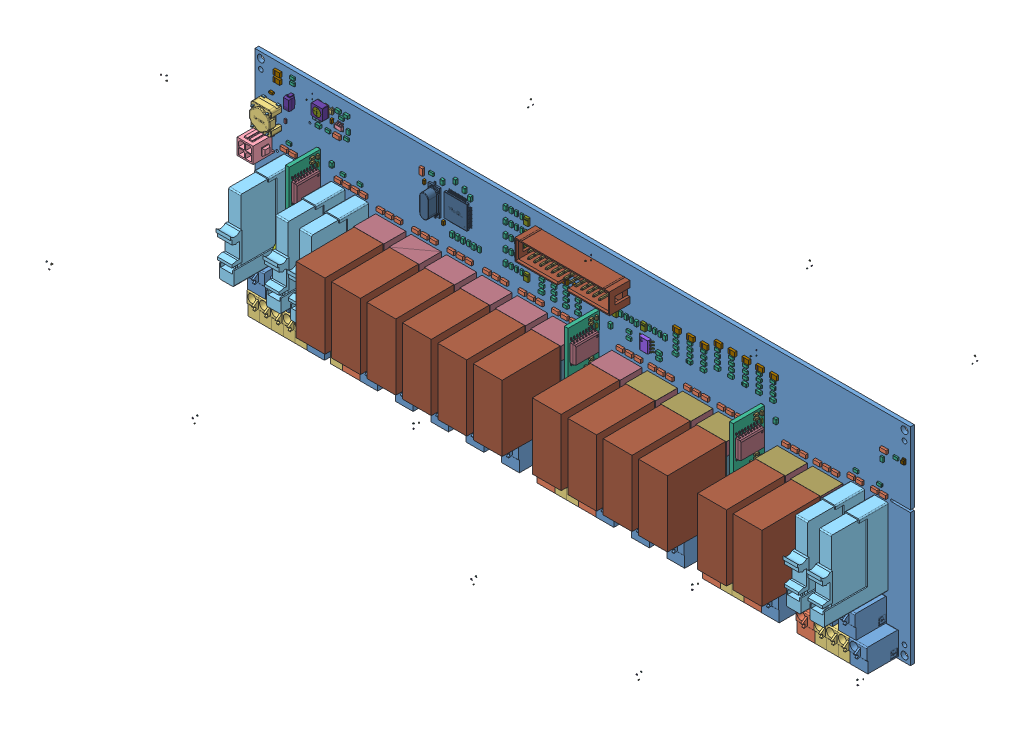
SolidWorks assembly _SC940D, configuration Default. Lengths in mm. (continued)
Components (placement in the parent): (continued)
- K11-1: K11 [Default] at origin size (13 30.3 34.5)
  - relais_40_61_8_006_0000-1: relais_40_61_8_006_0000 [Default] at (169.545 15.6766 9.5) x (0 1 0) z (1 0 0) size (29 30 12.4)
  - 1151724792-1: 1151724792 [Default] at (169.545 21.78 0) size (13 14.8 9.5)
    - Extruded_2-1: Extruded_2 [Default] at origin size (13 14.8 9.5)
  - 1151724928-1: 1151724928 [Default] at (169.545 41.93 0) size (13 5.5 9.5)
    - Extruded_3-1: Extruded_3 [Default] at origin size (13 5.5 9.5)
  - 1151725064-1: 1151725064 [Default] at (169.545 34.18 5) size (13 10 4.5)
    - Extruded_4-1: Extruded_4 [Default] at origin size (13 10 4.5)
- K14-1: K14 [Default] at origin size (13 30.3 34.5)
  - relais_40_61_8_006_0000-1: relais_40_61_8_006_0000 [Default] at (225.425 15.6766 9.5) x (0 1 0) z (1 0 0) size (29 30 12.4)
  - 1151724792-1: 1151724792 [Default] at (225.425 21.78 0) size (13 14.8 9.5)
    - Extruded_2-1: Extruded_2 [Default] at origin size (13 14.8 9.5)
  - 1151724928-1: 1151724928 [Default] at (225.425 41.93 0) size (13 5.5 9.5)
    - Extruded_3-1: Extruded_3 [Default] at origin size (13 5.5 9.5)
  - 1151725064-1: 1151725064 [Default] at (225.425 34.18 5) size (13 10 4.5)
    - Extruded_4-1: Extruded_4 [Default] at origin size (13 10 4.5)
- K15-1: K15 [Default] at origin size (13 30.3 34.5)
  - relais_40_61_8_006_0000-1: relais_40_61_8_006_0000 [Default] at (240.665 15.6766 9.5) x (0 1 0) z (1 0 0) size (29 30 12.4)
  - 1151724792-1: 1151724792 [Default] at (240.665 21.78 0) size (13 14.8 9.5)
    - Extruded_2-1: Extruded_2 [Default] at origin size (13 14.8 9.5)
  - 1151724928-1: 1151724928 [Default] at (240.665 41.93 0) size (13 5.5 9.5)
    - Extruded_3-1: Extruded_3 [Default] at origin size (13 5.5 9.5)
  - 1151725064-1: 1151725064 [Default] at (240.665 34.18 5) size (13 10 4.5)
    - Extruded_4-1: Extruded_4 [Default] at origin size (13 10 4.5)
- K1-1: K1 [Default] at origin size (6.2 33 32.7)
  - User_Library-93_11-1: User_Library-93_11 [Default] at (6.425 47.3038 0) x (0 -1 0) z (0 0 1) size (33 6.2 32.7)
- K2-1: K2 [Default] at origin size (6.2 33 32.7)
  - User_Library-93_11-1: User_Library-93_11 [Default] at (26.745 47.3038 0) x (0 -1 0) z (0 0 1) size (33 6.2 32.7)
- K3-1: K3 [Default] at origin size (6.2 33 32.7)
  - User_Library-93_11-1: User_Library-93_11 [Default] at (36.905 47.3038 0) x (0 -1 0) z (0 0 1) size (33 6.2 32.7)
- K16-1: K16 [Default] at origin size (6.2 33 32.7)
  - User_Library-93_11-1: User_Library-93_11 [Default] at (250.265 47.3038 0) x (0 -1 0) z (0 0 1) size (33 6.2 32.7)
- K17-1: K17 [Default] at origin size (6.2 33 32.7)
  - User_Library-93_11-1: User_Library-93_11 [Default] at (260.425 47.3038 0) x (0 -1 0) z (0 0 1) size (33 6.2 32.7)
- R45-1: R45 [Default] at origin size (2 1.2 0.7)
  - RESC2012X70N-1: RESC2012X70N [Default] at (155.5749 55.7212 0) x (-1 0 0) z (0 1 0) size (2 0.7 1.2)
- R46-1: R46 [Default] at origin size (2 1.2 0.7)
  - RESC2012X70N-1: RESC2012X70N [Default] at (155.5749 53.1812 0) x (-1 0 0) z (0 1 0) size (2 0.7 1.2)
- R34-1: R34 [Default] at origin size (1.2 2 0.7)
  - RESC2012X70N-1: RESC2012X70N [Default] at (109.4741 59.9439 0) x (0 -1 0) z (-1 0 0) size (2 0.7 1.2)
- R12_1-1: R12_1 [Default] at origin size (2 1.2 0.7)
  - RESC2012X70N-1: RESC2012X70N [Default] at (118.1099 58.6739 0) x (-1 0 0) z (0 1 0) size (2 0.7 1.2)
- R9_1-1: R9_1 [Default] at origin size (1.2 2 0.7)
  - RESC2012X70N-1: RESC2012X70N [Default] at (109.4741 70.3579 0) x (0 -1 0) z (-1 0 0) size (2 0.7 1.2)
- R16_1-1: R16_1 [Default] at origin size (1.2 2 0.7)
  - RESC2012X70N-1: RESC2012X70N [Default] at (109.4741 65.1509 0) x (0 -1 0) z (-1 0 0) size (2 0.7 1.2)
- R21-1: R21 [Default] at origin size (1.2 2 0.7)
  - RESC2012X70N-1: RESC2012X70N [Default] at (109.4741 75.5649 0) x (0 -1 0) z (-1 0 0) size (2 0.7 1.2)
- R27-1: R27 [Default] at origin size (1.2 2 0.7)
  - RESC2012X70N-1: RESC2012X70N [Default] at (109.4741 54.7369 0) x (0 -1 0) z (-1 0 0) size (2 0.7 1.2)
- R10-1: R10 [Default] at origin size (1.2 2 0.7)
  - RESC2012X70N-1: RESC2012X70N [Default] at (104.9021 70.3579 0) x (0 -1 0) z (-1 0 0) size (2 0.7 1.2)
- R15_1-1: R15_1 [Default] at origin size (1.2 2 0.7)
  - RESC2012X70N-1: RESC2012X70N [Default] at (104.9021 65.1509 0) x (0 -1 0) z (-1 0 0) size (2 0.7 1.2)
- R22-1: R22 [Default] at origin size (1.2 2 0.7)
  - RESC2012X70N-1: RESC2012X70N [Default] at (104.9021 75.5649 0) x (0 -1 0) z (-1 0 0) size (2 0.7 1.2)
- R28-1: R28 [Default] at origin size (1.2 2 0.7)
  - RESC2012X70N-1: RESC2012X70N [Default] at (104.9021 54.7369 0) x (0 -1 0) z (-1 0 0) size (2 0.7 1.2)
- R25_1-1: R25_1 [Default] at origin size (2 1.2 0.7)
  - RESC2012X70N-1: RESC2012X70N [Default] at (123.3169 54.1019 0) x (-1 0 0) z (0 1 0) size (2 0.7 1.2)
- R47-1: R47 [Default] at origin size (1.2 2 0.7)
  - RESC2012X70N-1: RESC2012X70N [Default] at (168.9101 61.4679 0) x (0 -1 0) z (-1 0 0) size (2 0.7 1.2)
- R18_1-1: R18_1 [Default] at origin size (2 1.2 0.7)
  - RESC2012X70N-1: RESC2012X70N [Default] at (128.5239 58.6739 0) x (-1 0 0) z (0 1 0) size (2 0.7 1.2)
- R24-1: R24 [Default] at origin size (2 1.2 0.7)
  - RESC2012X70N-1: RESC2012X70N [Default] at (123.3169 58.6739 0) x (-1 0 0) z (0 1 0) size (2 0.7 1.2)
- R33-1: R33 [Default] at origin size (1.2 2 0.7)
  - RESC2012X70N-1: RESC2012X70N [Default] at (104.9021 59.9439 0) x (0 -1 0) z (-1 0 0) size (2 0.7 1.2)
- R13-1: R13 [Default] at origin size (2 1.2 0.7)
  - RESC2012X70N-1: RESC2012X70N [Default] at (118.1099 54.1019 0) x (-1 0 0) z (0 1 0) size (2 0.7 1.2)
- R19_1-1: R19_1 [Default] at origin size (2 1.2 0.7)
  - RESC2012X70N-1: RESC2012X70N [Default] at (128.5239 54.1019 0) x (-1 0 0) z (0 1 0) size (2 0.7 1.2)
- R35-1: R35 [Default] at origin size (1.2 2 0.7)
  - RESC2012X70N-1: RESC2012X70N [Default] at (107.1879 59.9441 0) x (0 1 0) z (1 0 0) size (2 0.7 1.2)
- R14-1: R14 [Default] at origin size (2 1.2 0.7)
  - RESC2012X70N-1: RESC2012X70N [Default] at (118.1101 56.3881 0) x (1 0 0) z (0 -1 0) size (2 0.7 1.2)
- R20-1: R20 [Default] at origin size (2 1.2 0.7)
  - RESC2012X70N-1: RESC2012X70N [Default] at (128.5241 56.3881 0) x (1 0 0) z (0 -1 0) size (2 0.7 1.2)
- R31-1: R31 [Default] at origin size (2 1.2 0.7)
  - RESC2012X70N-1: RESC2012X70N [Default] at (133.7309 58.6739 0) x (-1 0 0) z (0 1 0) size (2 0.7 1.2)
- R36-1: R36 [Default] at origin size (1.2 2 0.7)
  - RESC2012X70N-1: RESC2012X70N [Default] at (139.7001 60.5789 0) x (0 -1 0) z (-1 0 0) size (2 0.7 1.2)
- R44-1: R44 [Default] at origin size (1.2 2 0.7)
  - RESC2012X70N-1: RESC2012X70N [Default] at (152.0191 60.5789 0) x (0 -1 0) z (-1 0 0) size (2 0.7 1.2)
- R49-1: R49 [Default] at origin size (1.2 2 0.7)
  - RESC2012X70N-1: RESC2012X70N [Default] at (164.3381 61.4679 0) x (0 -1 0) z (-1 0 0) size (2 0.7 1.2)
- R30-1: R30 [Default] at origin size (2 1.2 0.7)
  - RESC2012X70N-1: RESC2012X70N [Default] at (133.7309 54.1019 0) x (-1 0 0) z (0 1 0) size (2 0.7 1.2)
- R37-1: R37 [Default] at origin size (1.2 2 0.7)
  - RESC2012X70N-1: RESC2012X70N [Default] at (144.2721 60.5789 0) x (0 -1 0) z (-1 0 0) size (2 0.7 1.2)
- R42-1: R42 [Default] at origin size (1.2 2 0.7)
  - RESC2012X70N-1: RESC2012X70N [Default] at (156.5911 60.5789 0) x (0 -1 0) z (-1 0 0) size (2 0.7 1.2)
- R32-1: R32 [Default] at origin size (2 1.2 0.7)
  - RESC2012X70N-1: RESC2012X70N [Default] at (133.7311 56.3881 0) x (1 0 0) z (0 -1 0) size (2 0.7 1.2)
- R38-1: R38 [Default] at origin size (1.2 2 0.7)
  - RESC2012X70N-1: RESC2012X70N [Default] at (141.9859 60.5791 0) x (0 1 0) z (1 0 0) size (2 0.7 1.2)
- R43-1: R43 [Default] at origin size (1.2 2 0.7)
  - RESC2012X70N-1: RESC2012X70N [Default] at (154.3049 60.5791 0) x (0 1 0) z (1 0 0) size (2 0.7 1.2)
- R55-1: R55 [Default] at origin size (2 1.2 0.7)
  - RESC2012X70N-1: RESC2012X70N [Default] at (217.5511 68.0721 0) x (1 0 0) z (0 -1 0) size (2 0.7 1.2)
- R58-1: R58 [Default] at origin size (2 1.2 0.7)
  - RESC2012X70N-1: RESC2012X70N [Default] at (211.5821 68.0721 0) x (1 0 0) z (0 -1 0) size (2 0.7 1.2)
- R61-1: R61 [Default] at origin size (2 1.2 0.7)
  - RESC2012X70N-1: RESC2012X70N [Default] at (181.7371 64.5161 0) x (1 0 0) z (0 -1 0) size (2 0.7 1.2)
- R50-1: R50 [Default] at origin size (2 1.2 0.7)
  - RESC2012X70N-1: RESC2012X70N [Default] at (175.7681 59.9441 0) x (1 0 0) z (0 -1 0) size (2 0.7 1.2)
- R53-1: R53 [Default] at origin size (2 1.2 0.7)
  - RESC2012X70N-1: RESC2012X70N [Default] at (217.5511 63.5001 0) x (1 0 0) z (0 -1 0) size (2 0.7 1.2)
- R56-1: R56 [Default] at origin size (2 1.2 0.7)
  - RESC2012X70N-1: RESC2012X70N [Default] at (211.5821 63.5001 0) x (1 0 0) z (0 -1 0) size (2 0.7 1.2)
- R51-1: R51 [Default] at origin size (2 1.2 0.7)
  - RESC2012X70N-1: RESC2012X70N [Default] at (175.7679 62.2299 0) x (-1 0 0) z (0 1 0) size (2 0.7 1.2)
- R54-1: R54 [Default] at origin size (2 1.2 0.7)
  - RESC2012X70N-1: RESC2012X70N [Default] at (217.5509 65.7859 0) x (-1 0 0) z (0 1 0) size (2 0.7 1.2)
- R57-1: R57 [Default] at origin size (2 1.2 0.7)
  - RESC2012X70N-1: RESC2012X70N [Default] at (211.5819 65.7859 0) x (-1 0 0) z (0 1 0) size (2 0.7 1.2)
- R60-1: R60 [Default] at origin size (2 1.2 0.7)
  - RESC2012X70N-1: RESC2012X70N [Default] at (181.7369 62.2299 0) x (-1 0 0) z (0 1 0) size (2 0.7 1.2)
- R64-1: R64 [Default] at origin size (2 1.2 0.7)
  - RESC2012X70N-1: RESC2012X70N [Default] at (205.6131 68.0721 0) x (1 0 0) z (0 -1 0) size (2 0.7 1.2)
- R67-1: R67 [Default] at origin size (2 1.2 0.7)
  - RESC2012X70N-1: RESC2012X70N [Default] at (187.7061 64.5161 0) x (1 0 0) z (0 -1 0) size (2 0.7 1.2)
- R70-1: R70 [Default] at origin size (2 1.2 0.7)
  - RESC2012X70N-1: RESC2012X70N [Default] at (199.6441 68.0721 0) x (1 0 0) z (0 -1 0) size (2 0.7 1.2)
- R73-1: R73 [Default] at origin size (2 1.2 0.7)
  - RESC2012X70N-1: RESC2012X70N [Default] at (193.6751 68.0721 0) x (1 0 0) z (0 -1 0) size (2 0.7 1.2)
- R62-1: R62 [Default] at origin size (2 1.2 0.7)
  - RESC2012X70N-1: RESC2012X70N [Default] at (205.6131 63.5001 0) x (1 0 0) z (0 -1 0) size (2 0.7 1.2)
- R65-1: R65 [Default] at origin size (2 1.2 0.7)
  - RESC2012X70N-1: RESC2012X70N [Default] at (187.7061 59.9281 0) x (1 0 0) z (0 -1 0) size (2 0.7 1.2)
- R71-1: R71 [Default] at origin size (2 1.2 0.7)
  - RESC2012X70N-1: RESC2012X70N [Default] at (193.6751 63.5001 0) x (1 0 0) z (0 -1 0) size (2 0.7 1.2)
- R63-1: R63 [Default] at origin size (2 1.2 0.7)
  - RESC2012X70N-1: RESC2012X70N [Default] at (205.6129 65.7859 0) x (-1 0 0) z (0 1 0) size (2 0.7 1.2)
- R69-1: R69 [Default] at origin size (2 1.2 0.7)
  - RESC2012X70N-1: RESC2012X70N [Default] at (199.6439 65.7859 0) x (-1 0 0) z (0 1 0) size (2 0.7 1.2)
- R11_1-1: R11_1 [Default] at origin size (1.2 2 0.7)
  - RESC2012X70N-1: RESC2012X70N [Default] at (107.1879 70.3581 0) x (0 1 0) z (1 0 0) size (2 0.7 1.2)
- R17_1-1: R17_1 [Default] at origin size (1.2 2 0.7)
  - RESC2012X70N-1: RESC2012X70N [Default] at (107.1879 65.1511 0) x (0 1 0) z (1 0 0) size (2 0.7 1.2)
- R23-1: R23 [Default] at origin size (1.2 2 0.7)
  - RESC2012X70N-1: RESC2012X70N [Default] at (107.1879 75.5651 0) x (0 1 0) z (1 0 0) size (2 0.7 1.2)
- R29-1: R29 [Default] at origin size (1.2 2 0.7)
  - RESC2012X70N-1: RESC2012X70N [Default] at (107.1879 54.7371 0) x (0 1 0) z (1 0 0) size (2 0.7 1.2)
- R26_1-1: R26_1 [Default] at origin size (2 1.2 0.7)
  - RESC2012X70N-1: RESC2012X70N [Default] at (123.3171 56.3881 0) x (1 0 0) z (0 -1 0) size (2 0.7 1.2)
- R48-1: R48 [Default] at origin size (1.2 2 0.7)
  - RESC2012X70N-1: RESC2012X70N [Default] at (166.6239 61.4681 0) x (0 1 0) z (1 0 0) size (2 0.7 1.2)
- R72-1: R72 [Default] at origin size (2 1.2 0.7)
  - RESC2012X70N-1: RESC2012X70N [Default] at (193.6749 65.7859 0) x (-1 0 0) z (0 1 0) size (2 0.7 1.2)
- R1_1-1: R1_1 [Default] at origin size (2 1.2 0.7)
  - RESC2012X70N-1: RESC2012X70N [Default] at (10.8267 77.7717 0) x (-1 0 0) z (0 1 0) size (2 0.7 1.2)
- R2_1-1: R2_1 [Default] at origin size (2 1.2 0.7)
  - RESC2012X70N-1: RESC2012X70N [Default] at (10.8267 75.7079 0) x (-1 0 0) z (0 1 0) size (2 0.7 1.2)
- R76-1: R76 [Default] at origin size (1.2 2 0.7)
  - RESC2012X70N-1: RESC2012X70N [Default] at (264.4776 62.7062 0) x (0 -1 0) z (-1 0 0) size (2 0.7 1.2)
- R41-1: R41 [Default] at origin size (1.2 2 0.7)
  - RESC2012X70N-1: RESC2012X70N [Default] at (86.6141 54.1019 0) x (0 -1 0) z (-1 0 0) size (2 0.7 1.2)
- R40-1: R40 [Default] at origin size (1.2 2 0.7)
  - RESC2012X70N-1: RESC2012X70N [Default] at (91.1861 54.1019 0) x (0 -1 0) z (-1 0 0) size (2 0.7 1.2)
- R39-1: R39 [Default] at origin size (2 1.2 0.7)
  - RESC2012X70N-1: RESC2012X70N [Default] at (70.6121 72.1361 0) x (1 0 0) z (0 -1 0) size (2 0.7 1.2)
- R77-1: R77 [Default] at origin size (2 1.2 0.7)
  - RESC2012X70N-1: RESC2012X70N [Default] at (270.3513 66.0401 0) x (1 0 0) z (0 -1 0) size (2 0.7 1.2)
- SUP_K4-1: SUP_K4 [Default] at origin size (13 30.3 9.5)
  - 1151724792-1: 1151724792 [Default] at (52.705 21.825 0) size (13 14.8 9.5)
    - Extruded_2-1: Extruded_2 [Default] at origin size (13 14.8 9.5)
  - 1151725064-1: 1151725064 [Default] at (52.705 34.225 5) size (13 10 4.5)
    - Extruded_4-1: Extruded_4 [Default] at origin size (13 10 4.5)
  - 1151724928-1: 1151724928 [Default] at (52.705 41.975 0) size (13 5.5 9.5)
    - Extruded_3-1: Extruded_3 [Default] at origin size (13 5.5 9.5)
- SUP_K5-1: SUP_K5 [Default] at origin size (13 30.3 9.5)
  - 1151724792-1: 1151724792 [Default] at (67.945 21.825 0) size (13 14.8 9.5)
    - Extruded_2-1: Extruded_2 [Default] at origin size (13 14.8 9.5)
  - 1151725064-1: 1151725064 [Default] at (67.945 34.225 5) size (13 10 4.5)
    - Extruded_4-1: Extruded_4 [Default] at origin size (13 10 4.5)
  - 1151724928-1: 1151724928 [Default] at (67.945 41.975 0) size (13 5.5 9.5)
    - Extruded_3-1: Extruded_3 [Default] at origin size (13 5.5 9.5)
- SUP_K6-1: SUP_K6 [Default] at origin size (13 30.3 9.5)
  - 1151724792-1: 1151724792 [Default] at (83.185 21.825 0) size (13 14.8 9.5)
    - Extruded_2-1: Extruded_2 [Default] at origin size (13 14.8 9.5)
  - 1151725064-1: 1151725064 [Default] at (83.185 34.225 5) size (13 10 4.5)
    - Extruded_4-1: Extruded_4 [Default] at origin size (13 10 4.5)
  - 1151724928-1: 1151724928 [Default] at (83.185 41.975 0) size (13 5.5 9.5)
    - Extruded_3-1: Extruded_3 [Default] at origin size (13 5.5 9.5)
- SUP_K7-1: SUP_K7 [Default] at origin size (13 30.3 9.5)
  - 1151724792-1: 1151724792 [Default] at (98.425 21.825 0) size (13 14.8 9.5)
    - Extruded_2-1: Extruded_2 [Default] at origin size (13 14.8 9.5)
  - 1151725064-1: 1151725064 [Default] at (98.425 34.225 5) size (13 10 4.5)
    - Extruded_4-1: Extruded_4 [Default] at origin size (13 10 4.5)
  - 1151724928-1: 1151724928 [Default] at (98.425 41.975 0) size (13 5.5 9.5)
    - Extruded_3-1: Extruded_3 [Default] at origin size (13 5.5 9.5)
- SUP_K8-1: SUP_K8 [Default] at origin size (13 30.3 9.5)
  - 1151724792-1: 1151724792 [Default] at (113.665 21.825 0) size (13 14.8 9.5)
    - Extruded_2-1: Extruded_2 [Default] at origin size (13 14.8 9.5)
  - 1151725064-1: 1151725064 [Default] at (113.665 34.225 5) size (13 10 4.5)
    - Extruded_4-1: Extruded_4 [Default] at origin size (13 10 4.5)
  - 1151724928-1: 1151724928 [Default] at (113.665 41.975 0) size (13 5.5 9.5)
    - Extruded_3-1: Extruded_3 [Default] at origin size (13 5.5 9.5)
- SUP_K9-1: SUP_K9 [Default] at origin size (13 30.3 9.5)
  - 1151724792-1: 1151724792 [Default] at (128.905 21.825 0) size (13 14.8 9.5)
    - Extruded_2-1: Extruded_2 [Default] at origin size (13 14.8 9.5)
  - 1151725064-1: 1151725064 [Default] at (128.905 34.225 5) size (13 10 4.5)
    - Extruded_4-1: Extruded_4 [Default] at origin size (13 10 4.5)
  - 1151724928-1: 1151724928 [Default] at (128.905 41.975 0) size (13 5.5 9.5)
    - Extruded_3-1: Extruded_3 [Default] at origin size (13 5.5 9.5)
- SUP_K10-1: SUP_K10 [Default] at origin size (13 30.3 9.5)
  - 1151724792-1: 1151724792 [Default] at (154.305 21.825 0) size (13 14.8 9.5)
    - Extruded_2-1: Extruded_2 [Default] at origin size (13 14.8 9.5)
  - 1151725064-1: 1151725064 [Default] at (154.305 34.225 5) size (13 10 4.5)
    - Extruded_4-1: Extruded_4 [Default] at origin size (13 10 4.5)
  - 1151724928-1: 1151724928 [Default] at (154.305 41.975 0) size (13 5.5 9.5)
    - Extruded_3-1: Extruded_3 [Default] at origin size (13 5.5 9.5)
- SUP_K11-1: SUP_K11 [Default] at origin size (13 30.3 9.5)
  - 1151724792-1: 1151724792 [Default] at (169.545 37.325 0) size (13 14.8 9.5)
    - Extruded_2-1: Extruded_2 [Default] at origin size (13 14.8 9.5)
  - 1151725064-1: 1151725064 [Default] at (169.545 24.925 5) size (13 10 4.5)
    - Extruded_4-1: Extruded_4 [Default] at origin size (13 10 4.5)
  - 1151724928-1: 1151724928 [Default] at (169.545 17.175 0) size (13 5.5 9.5)
    - Extruded_3-1: Extruded_3 [Default] at origin size (13 5.5 9.5)
- SUP_K14-1: SUP_K14 [Default] at origin size (13 30.3 9.5)
  - 1151724792-1: 1151724792 [Default] at (225.425 37.325 0) size (13 14.8 9.5)
    - Extruded_2-1: Extruded_2 [Default] at origin size (13 14.8 9.5)
  - 1151725064-1: 1151725064 [Default] at (225.425 24.925 5) size (13 10 4.5)
    - Extruded_4-1: Extruded_4 [Default] at origin size (13 10 4.5)
  - 1151724928-1: 1151724928 [Default] at (225.425 17.175 0) size (13 5.5 9.5)
    - Extruded_3-1: Extruded_3 [Default] at origin size (13 5.5 9.5)
- SUP_K15-1: SUP_K15 [Default] at origin size (13 30.3 9.5)
  - 1151724792-1: 1151724792 [Default] at (240.665 37.325 0) size (13 14.8 9.5)
    - Extruded_2-1: Extruded_2 [Default] at origin size (13 14.8 9.5)
  - 1151725064-1: 1151725064 [Default] at (240.665 24.925 5) size (13 10 4.5)
    - Extruded_4-1: Extruded_4 [Default] at origin size (13 10 4.5)
  - 1151724928-1: 1151724928 [Default] at (240.665 17.175 0) size (13 5.5 9.5)
    - Extruded_3-1: Extruded_3 [Default] at origin size (13 5.5 9.5)
- T30-1: T30 [Default] at origin size (196.44 46.45 23.48)
  - SW3dPS-transistor_SOT233_4-1: SW3dPS-transistor_SOT233_4 [Default] at (193.1288 43.5744 -21.9) x (-1 0 0) z (0 1 0) size (2.9 1.1 1.6)
  - SW3dPS-transistor_SOT233_5-1: SW3dPS-transistor_SOT233_5 [Default] at (0.1931 0.0436 -0.0219) x (-1 0 0) z (0 1 0) size (2.18 2.18 2.18)
  - SW3dPS-transistor_SOT233_6-1: SW3dPS-transistor_SOT233_6 [Default] at (0.0002 0 0) x (-1 0 0) z (0 1 0) size (2.18 2.18 2.18)
  - SW3dPS-transistor_SOT233_7-1: SW3dPS-transistor_SOT233_7 [Default] x (-1 0 0) z (0 1 0) size (2.18 2.18 2.18)
- U6-1: U6 [Default] at origin size (6.2 5 1.75)
  - User_Library-SOIC-8-150_1-1: User_Library-SOIC-8-150_1 [Default] at (163.0363 55.0862 1) x (0 1 0) z (1 0 0) size (5 1.75 6.2)
    - User_Library-SOIC-8-150_pin_SOIC_SO-150_1-1: User_Library-SOIC-8-150_pin_SOIC_SO-150_1 [Default] at (0.6 0 -2) x (-1 0 0) z (0 0 -1) size (0.4 1.1 1.1)
    - User_Library-SOIC-8-150_pin_SOIC_SO-150_1-2: User_Library-SOIC-8-150_pin_SOIC_SO-150_1 [Default] at (-0.67 0 -2) x (-1 0 0) z (0 0 -1) size (0.4 1.1 1.1)
    - User_Library-SOIC-8-150_pin_SOIC_SO-150_1-3: User_Library-SOIC-8-150_pin_SOIC_SO-150_1 [Default] at (-1.94 0 2) size (0.4 1.1 1.1)
    - User_Library-SOIC-8-150_pin_SOIC_SO-150_1-4: User_Library-SOIC-8-150_pin_SOIC_SO-150_1 [Default] at (-0.67 0 2) size (0.4 1.1 1.1)
    - User_Library-SOIC-8-150_pin_SOIC_SO-150_1-5: User_Library-SOIC-8-150_pin_SOIC_SO-150_1 [Default] at (-1.94 0 -2) x (-1 0 0) z (0 0 -1) size (0.4 1.1 1.1)
    - User_Library-SOIC-8-150_pin_SOIC_SO-150_1-6: User_Library-SOIC-8-150_pin_SOIC_SO-150_1 [Default] at (1.87 0 2) size (0.4 1.1 1.1)
    - User_Library-SOIC-8-150_SOIC_150_SOIC_5X4_1-1: User_Library-SOIC-8-150_SOIC_150_SOIC_5X4_1 [Default] at origin size (5 1.5 4)
    - User_Library-SOIC-8-150_pin_SOIC_SO-150_1-7: User_Library-SOIC-8-150_pin_SOIC_SO-150_1 [Default] at (0.6 0 2) size (0.4 1.1 1.1)
    - User_Library-SOIC-8-150_pin_SOIC_SO-150_1-8: User_Library-SOIC-8-150_pin_SOIC_SO-150_1 [Default] at (1.87 0 -2) x (-1 0 0) z (0 0 -1) size (0.4 1.1 1.1)
- U3-1: U3 [Default] at origin size (92.36 4.66 23.48)
  - SW3dPS-transistor_SOT233_4-1: SW3dPS-transistor_SOT233_4 [Default] at (89.4898 -1.1812 -21.9) x (0 -1 0) z (-1 0 0) size (2.9 1.1 1.6)
  - SW3dPS-transistor_SOT233_5-1: SW3dPS-transistor_SOT233_5 [Default] at (0.0895 -0.0012 -0.0219) x (0 -1 0) z (-1 0 0) size (2.18 2.18 2.18)
  - SW3dPS-transistor_SOT233_6-1: SW3dPS-transistor_SOT233_6 [Default] at (0.0001 0 0) x (0 -1 0) z (-1 0 0) size (2.18 2.18 2.18)
  - SW3dPS-transistor_SOT233_7-1: SW3dPS-transistor_SOT233_7 [Default] x (0 -1 0) z (-1 0 0) size (2.18 2.18 2.18)
- D8-1: D8 [Default] at origin size (41.49 29.62 23.48)
  - SW3dPS-transistor_SOT233_4-1: SW3dPS-transistor_SOT233_4 [Default] at (-38.0112 26.7469 -21.9) x (-1 0 0) z (0 1 0) size (2.9 1.1 1.6)
  - SW3dPS-transistor_SOT233_5-1: SW3dPS-transistor_SOT233_5 [Default] at (-0.038 0.0267 -0.0219) x (-1 0 0) z (0 1 0) size (2.18 2.18 2.18)
  - SW3dPS-transistor_SOT233_6-1: SW3dPS-transistor_SOT233_6 [Default] at (0 0 0) x (-1 0 0) z (0 1 0) size (2.18 2.18 2.18)
  - SW3dPS-transistor_SOT233_7-1: SW3dPS-transistor_SOT233_7 [Default] x (-1 0 0) z (0 1 0) size (2.18 2.18 2.18)
- R7_1-1: R7_1 [Default] at origin size (2 1.2 0.7)
  - RESC2012X70N-1: RESC2012X70N [Default] at (32.5437 52.7049 0) x (-1 0 0) z (0 1 0) size (2 0.7 1.2)
- T2-1: T2 [Default] at origin size (106.42 75.5 23.48)
  - SW3dPS-transistor_SOT233_4-1: SW3dPS-transistor_SOT233_4 [Default] at (102.9399 72.6306 -21.9) x (1 0 0) z (0 -1 0) size (2.9 1.1 1.6)
  - SW3dPS-transistor_SOT233_5-1: SW3dPS-transistor_SOT233_5 [Default] at (0.1029 0.0726 -0.0219) x (1 0 0) z (0 -1 0) size (2.18 2.18 2.18)
  - SW3dPS-transistor_SOT233_6-1: SW3dPS-transistor_SOT233_6 [Default] at (0.0001 0.0001 0) x (1 0 0) z (0 -1 0) size (2.18 2.18 2.18)
  - SW3dPS-transistor_SOT233_7-1: SW3dPS-transistor_SOT233_7 [Default] x (1 0 0) z (0 -1 0) size (2.18 2.18 2.18)
- D9-1: D9 [Default] at origin size (34.19 29.62 23.48)
  - SW3dPS-transistor_SOT233_4-1: SW3dPS-transistor_SOT233_4 [Default] at (-30.7087 26.7469 -21.9) x (-1 0 0) z (0 1 0) size (2.9 1.1 1.6)
  - SW3dPS-transistor_SOT233_5-1: SW3dPS-transistor_SOT233_5 [Default] at (-0.0307 0.0267 -0.0219) x (-1 0 0) z (0 1 0) size (2.18 2.18 2.18)
  - SW3dPS-transistor_SOT233_6-1: SW3dPS-transistor_SOT233_6 [Default] at (0 0 0) x (-1 0 0) z (0 1 0) size (2.18 2.18 2.18)
  - SW3dPS-transistor_SOT233_7-1: SW3dPS-transistor_SOT233_7 [Default] x (-1 0 0) z (0 1 0) size (2.18 2.18 2.18)
- R8_1-1: R8_1 [Default] at origin size (2 1.2 0.7)
  - RESC2012X70N-1: RESC2012X70N [Default] at (39.8462 52.7049 0) x (-1 0 0) z (0 1 0) size (2 0.7 1.2)
- T3_1-1: T3_1 [Default] at origin size (113.72 75.5 23.48)
  - SW3dPS-transistor_SOT233_4-1: SW3dPS-transistor_SOT233_4 [Default] at (110.2424 72.6306 -21.9) x (1 0 0) z (0 -1 0) size (2.9 1.1 1.6)
  - SW3dPS-transistor_SOT233_5-1: SW3dPS-transistor_SOT233_5 [Default] at (0.1102 0.0726 -0.0219) x (1 0 0) z (0 -1 0) size (2.18 2.18 2.18)
  - SW3dPS-transistor_SOT233_6-1: SW3dPS-transistor_SOT233_6 [Default] at (0.0001 0.0001 0) x (1 0 0) z (0 -1 0) size (2.18 2.18 2.18)
  - SW3dPS-transistor_SOT233_7-1: SW3dPS-transistor_SOT233_7 [Default] x (1 0 0) z (0 -1 0) size (2.18 2.18 2.18)
- D11-1: D11 [Default] at origin size (23.07 27.55 23.48)
  - SW3dPS-transistor_SOT233_4-1: SW3dPS-transistor_SOT233_4 [Default] at (-19.5962 24.6832 -21.9) x (-1 0 0) z (0 1 0) size (2.9 1.1 1.6)
  - SW3dPS-transistor_SOT233_5-1: SW3dPS-transistor_SOT233_5 [Default] at (-0.0196 0.0247 -0.0219) x (-1 0 0) z (0 1 0) size (2.18 2.18 2.18)
  - SW3dPS-transistor_SOT233_6-1: SW3dPS-transistor_SOT233_6 [Default] at (0 0 0) x (-1 0 0) z (0 1 0) size (2.18 2.18 2.18)
  - SW3dPS-transistor_SOT233_7-1: SW3dPS-transistor_SOT233_7 [Default] x (-1 0 0) z (0 1 0) size (2.18 2.18 2.18)
- T5_1-1: T5_1 [Default] at origin size (132.29 73.44 23.48)
  - SW3dPS-transistor_SOT233_4-1: SW3dPS-transistor_SOT233_4 [Default] at (128.8162 70.5668 -21.9) x (1 0 0) z (0 -1 0) size (2.9 1.1 1.6)
  - SW3dPS-transistor_SOT233_5-1: SW3dPS-transistor_SOT233_5 [Default] at (0.1288 0.0706 -0.0219) x (1 0 0) z (0 -1 0) size (2.18 2.18 2.18)
  - SW3dPS-transistor_SOT233_6-1: SW3dPS-transistor_SOT233_6 [Default] at (0.0001 0.0001 0) x (1 0 0) z (0 -1 0) size (2.18 2.18 2.18)
  - SW3dPS-transistor_SOT233_7-1: SW3dPS-transistor_SOT233_7 [Default] x (1 0 0) z (0 -1 0) size (2.18 2.18 2.18)
- T4_1-1: T4_1 [Default] at origin size (124.67 73.44 23.48)
  - SW3dPS-transistor_SOT233_4-1: SW3dPS-transistor_SOT233_4 [Default] at (121.1962 70.5668 -21.9) x (1 0 0) z (0 -1 0) size (2.9 1.1 1.6)
  - SW3dPS-transistor_SOT233_5-1: SW3dPS-transistor_SOT233_5 [Default] at (0.1212 0.0706 -0.0219) x (1 0 0) z (0 -1 0) size (2.18 2.18 2.18)
  - SW3dPS-transistor_SOT233_6-1: SW3dPS-transistor_SOT233_6 [Default] at (0.0001 0.0001 0) x (1 0 0) z (0 -1 0) size (2.18 2.18 2.18)
  - SW3dPS-transistor_SOT233_7-1: SW3dPS-transistor_SOT233_7 [Default] x (1 0 0) z (0 -1 0) size (2.18 2.18 2.18)
- D15-1: D15 [Default] at origin size (7.83 27.55 23.48)
  - SW3dPS-transistor_SOT233_4-1: SW3dPS-transistor_SOT233_4 [Default] at (-4.3562 24.6832 -21.9) x (-1 0 0) z (0 1 0) size (2.9 1.1 1.6)
  - SW3dPS-transistor_SOT233_5-1: SW3dPS-transistor_SOT233_5 [Default] at (-0.0044 0.0247 -0.0219) x (-1 0 0) z (0 1 0) size (2.18 2.18 2.18)
  - SW3dPS-transistor_SOT233_6-1: SW3dPS-transistor_SOT233_6 [Default] at (0 0 0) x (-1 0 0) z (0 1 0) size (2.18 2.18 2.18)
  - SW3dPS-transistor_SOT233_7-1: SW3dPS-transistor_SOT233_7 [Default] x (-1 0 0) z (0 1 0) size (2.18 2.18 2.18)
- T7_1-1: T7_1 [Default] at origin size (147.53 73.44 23.48)
  - SW3dPS-transistor_SOT233_4-1: SW3dPS-transistor_SOT233_4 [Default] at (144.0562 70.5668 -21.9) x (1 0 0) z (0 -1 0) size (2.9 1.1 1.6)
  - SW3dPS-transistor_SOT233_5-1: SW3dPS-transistor_SOT233_5 [Default] at (0.1441 0.0706 -0.0219) x (1 0 0) z (0 -1 0) size (2.18 2.18 2.18)
  - SW3dPS-transistor_SOT233_6-1: SW3dPS-transistor_SOT233_6 [Default] at (0.0001 0.0001 0) x (1 0 0) z (0 -1 0) size (2.18 2.18 2.18)
  - SW3dPS-transistor_SOT233_7-1: SW3dPS-transistor_SOT233_7 [Default] x (1 0 0) z (0 -1 0) size (2.18 2.18 2.18)
- T6_1-1: T6_1 [Default] at origin size (139.91 73.44 23.48)
  - SW3dPS-transistor_SOT233_4-1: SW3dPS-transistor_SOT233_4 [Default] at (136.4362 70.5668 -21.9) x (1 0 0) z (0 -1 0) size (2.9 1.1 1.6)
  - SW3dPS-transistor_SOT233_5-1: SW3dPS-transistor_SOT233_5 [Default] at (0.1364 0.0706 -0.0219) x (1 0 0) z (0 -1 0) size (2.18 2.18 2.18)
  - SW3dPS-transistor_SOT233_6-1: SW3dPS-transistor_SOT233_6 [Default] at (0.0001 0.0001 0) x (1 0 0) z (0 -1 0) size (2.18 2.18 2.18)
  - SW3dPS-transistor_SOT233_7-1: SW3dPS-transistor_SOT233_7 [Default] x (1 0 0) z (0 -1 0) size (2.18 2.18 2.18)
- T9-1: T9 [Default] at origin size (162.77 73.44 23.48)
  - SW3dPS-transistor_SOT233_4-1: SW3dPS-transistor_SOT233_4 [Default] at (159.2962 70.5668 -21.9) x (1 0 0) z (0 -1 0) size (2.9 1.1 1.6)
  - SW3dPS-transistor_SOT233_5-1: SW3dPS-transistor_SOT233_5 [Default] at (0.1593 0.0706 -0.0219) x (1 0 0) z (0 -1 0) size (2.18 2.18 2.18)
  - SW3dPS-transistor_SOT233_6-1: SW3dPS-transistor_SOT233_6 [Default] at (0.0002 0.0001 0) x (1 0 0) z (0 -1 0) size (2.18 2.18 2.18)
  - SW3dPS-transistor_SOT233_7-1: SW3dPS-transistor_SOT233_7 [Default] x (1 0 0) z (0 -1 0) size (2.18 2.18 2.18)
- T8-1: T8 [Default] at origin size (155.15 73.44 23.48)
  - SW3dPS-transistor_SOT233_4-1: SW3dPS-transistor_SOT233_4 [Default] at (151.6762 70.5668 -21.9) x (1 0 0) z (0 -1 0) size (2.9 1.1 1.6)
  - SW3dPS-transistor_SOT233_5-1: SW3dPS-transistor_SOT233_5 [Default] at (0.1517 0.0706 -0.0219) x (1 0 0) z (0 -1 0) size (2.18 2.18 2.18)
  - SW3dPS-transistor_SOT233_6-1: SW3dPS-transistor_SOT233_6 [Default] at (0.0002 0.0001 0) x (1 0 0) z (0 -1 0) size (2.18 2.18 2.18)
  - SW3dPS-transistor_SOT233_7-1: SW3dPS-transistor_SOT233_7 [Default] x (1 0 0) z (0 -1 0) size (2.18 2.18 2.18)
- D23-1: D23 [Default] at origin size (29.6 27.55 23.48)
  - SW3dPS-transistor_SOT233_4-1: SW3dPS-transistor_SOT233_4 [Default] at (26.1238 24.6832 -21.9) x (-1 0 0) z (0 1 0) size (2.9 1.1 1.6)
  - SW3dPS-transistor_SOT233_5-1: SW3dPS-transistor_SOT233_5 [Default] at (0.0261 0.0247 -0.0219) x (-1 0 0) z (0 1 0) size (2.18 2.18 2.18)
  - SW3dPS-transistor_SOT233_6-1: SW3dPS-transistor_SOT233_6 [Default] at (0 0 0) x (-1 0 0) z (0 1 0) size (2.18 2.18 2.18)
  - SW3dPS-transistor_SOT233_7-1: SW3dPS-transistor_SOT233_7 [Default] x (-1 0 0) z (0 1 0) size (2.18 2.18 2.18)
- T11-1: T11 [Default] at origin size (178.01 73.44 23.48)
  - SW3dPS-transistor_SOT233_4-1: SW3dPS-transistor_SOT233_4 [Default] at (174.5362 70.5668 -21.9) x (1 0 0) z (0 -1 0) size (2.9 1.1 1.6)
  - SW3dPS-transistor_SOT233_5-1: SW3dPS-transistor_SOT233_5 [Default] at (0.1745 0.0706 -0.0219) x (1 0 0) z (0 -1 0) size (2.18 2.18 2.18)
  - SW3dPS-transistor_SOT233_6-1: SW3dPS-transistor_SOT233_6 [Default] at (0.0002 0.0001 0) x (1 0 0) z (0 -1 0) size (2.18 2.18 2.18)
  - SW3dPS-transistor_SOT233_7-1: SW3dPS-transistor_SOT233_7 [Default] x (1 0 0) z (0 -1 0) size (2.18 2.18 2.18)
- T10-1: T10 [Default] at origin size (170.39 73.44 23.48)
  - SW3dPS-transistor_SOT233_4-1: SW3dPS-transistor_SOT233_4 [Default] at (166.9162 70.5668 -21.9) x (1 0 0) z (0 -1 0) size (2.9 1.1 1.6)
  - SW3dPS-transistor_SOT233_5-1: SW3dPS-transistor_SOT233_5 [Default] at (0.1669 0.0706 -0.0219) x (1 0 0) z (0 -1 0) size (2.18 2.18 2.18)
  - SW3dPS-transistor_SOT233_6-1: SW3dPS-transistor_SOT233_6 [Default] at (0.0002 0.0001 0) x (1 0 0) z (0 -1 0) size (2.18 2.18 2.18)
  - SW3dPS-transistor_SOT233_7-1: SW3dPS-transistor_SOT233_7 [Default] x (1 0 0) z (0 -1 0) size (2.18 2.18 2.18)
- D24-1: D24 [Default] at origin size (44.82 27.55 23.48)
  - SW3dPS-transistor_SOT233_4-1: SW3dPS-transistor_SOT233_4 [Default] at (41.3638 24.6832 -21.9) x (-1 0 0) z (0 1 0) size (2.9 1.1 1.6)
  - SW3dPS-transistor_SOT233_5-1: SW3dPS-transistor_SOT233_5 [Default] at (0.0414 0.0247 -0.0219) x (-1 0 0) z (0 1 0) size (2.18 2.18 2.18)
  - SW3dPS-transistor_SOT233_6-1: SW3dPS-transistor_SOT233_6 [Default] at (0 0 0) x (-1 0 0) z (0 1 0) size (2.18 2.18 2.18)
  - SW3dPS-transistor_SOT233_7-1: SW3dPS-transistor_SOT233_7 [Default] x (-1 0 0) z (0 1 0) size (2.18 2.18 2.18)
- T13-1: T13 [Default] at origin size (193.25 73.44 23.48)
  - SW3dPS-transistor_SOT233_4-1: SW3dPS-transistor_SOT233_4 [Default] at (189.7762 70.5668 -21.9) x (1 0 0) z (0 -1 0) size (2.9 1.1 1.6)
  - SW3dPS-transistor_SOT233_5-1: SW3dPS-transistor_SOT233_5 [Default] at (0.1898 0.0706 -0.0219) x (1 0 0) z (0 -1 0) size (2.18 2.18 2.18)
  - SW3dPS-transistor_SOT233_6-1: SW3dPS-transistor_SOT233_6 [Default] at (0.0002 0.0001 0) x (1 0 0) z (0 -1 0) size (2.18 2.18 2.18)
  - SW3dPS-transistor_SOT233_7-1: SW3dPS-transistor_SOT233_7 [Default] x (1 0 0) z (0 -1 0) size (2.18 2.18 2.18)
- T12-1: T12 [Default] at origin size (185.63 73.44 23.48)
  - SW3dPS-transistor_SOT233_4-1: SW3dPS-transistor_SOT233_4 [Default] at (182.1562 70.5668 -21.9) x (1 0 0) z (0 -1 0) size (2.9 1.1 1.6)
  - SW3dPS-transistor_SOT233_5-1: SW3dPS-transistor_SOT233_5 [Default] at (0.1822 0.0706 -0.0219) x (1 0 0) z (0 -1 0) size (2.18 2.18 2.18)
  - SW3dPS-transistor_SOT233_6-1: SW3dPS-transistor_SOT233_6 [Default] at (0.0002 0.0001 0) x (1 0 0) z (0 -1 0) size (2.18 2.18 2.18)
  - SW3dPS-transistor_SOT233_7-1: SW3dPS-transistor_SOT233_7 [Default] x (1 0 0) z (0 -1 0) size (2.18 2.18 2.18)
- D25-1: D25 [Default] at origin size (59.26 27.55 23.48)
  - SW3dPS-transistor_SOT233_4-1: SW3dPS-transistor_SOT233_4 [Default] at (55.8101 24.6832 -21.9) x (-1 0 0) z (0 1 0) size (2.9 1.1 1.6)
  - SW3dPS-transistor_SOT233_5-1: SW3dPS-transistor_SOT233_5 [Default] at (0.0558 0.0247 -0.0219) x (-1 0 0) z (0 1 0) size (2.18 2.18 2.18)
  - SW3dPS-transistor_SOT233_6-1: SW3dPS-transistor_SOT233_6 [Default] at (0.0001 0 0) x (-1 0 0) z (0 1 0) size (2.18 2.18 2.18)
  - SW3dPS-transistor_SOT233_7-1: SW3dPS-transistor_SOT233_7 [Default] x (-1 0 0) z (0 1 0) size (2.18 2.18 2.18)
- T15-1: T15 [Default] at origin size (207.7 73.44 23.48)
  - SW3dPS-transistor_SOT233_4-1: SW3dPS-transistor_SOT233_4 [Default] at (204.2224 70.5668 -21.9) x (1 0 0) z (0 -1 0) size (2.9 1.1 1.6)
  - SW3dPS-transistor_SOT233_5-1: SW3dPS-transistor_SOT233_5 [Default] at (0.2042 0.0706 -0.0219) x (1 0 0) z (0 -1 0) size (2.18 2.18 2.18)
  - SW3dPS-transistor_SOT233_6-1: SW3dPS-transistor_SOT233_6 [Default] at (0.0002 0.0001 0) x (1 0 0) z (0 -1 0) size (2.18 2.18 2.18)
  - SW3dPS-transistor_SOT233_7-1: SW3dPS-transistor_SOT233_7 [Default] x (1 0 0) z (0 -1 0) size (2.18 2.18 2.18)
- T14-1: T14 [Default] at origin size (200.08 73.44 23.48)
  - SW3dPS-transistor_SOT233_4-1: SW3dPS-transistor_SOT233_4 [Default] at (196.6024 70.5668 -21.9) x (1 0 0) z (0 -1 0) size (2.9 1.1 1.6)
  - SW3dPS-transistor_SOT233_5-1: SW3dPS-transistor_SOT233_5 [Default] at (0.1966 0.0706 -0.0219) x (1 0 0) z (0 -1 0) size (2.18 2.18 2.18)
  - SW3dPS-transistor_SOT233_6-1: SW3dPS-transistor_SOT233_6 [Default] at (0.0002 0.0001 0) x (1 0 0) z (0 -1 0) size (2.18 2.18 2.18)
  - SW3dPS-transistor_SOT233_7-1: SW3dPS-transistor_SOT233_7 [Default] x (1 0 0) z (0 -1 0) size (2.18 2.18 2.18)
- D27-1: D27 [Default] at origin size (87.01 27.55 23.48)
  - SW3dPS-transistor_SOT233_4-1: SW3dPS-transistor_SOT233_4 [Default] at (83.5913 24.6832 -21.9) x (-1 0 0) z (0 1 0) size (2.9 1.1 1.6)
  - SW3dPS-transistor_SOT233_5-1: SW3dPS-transistor_SOT233_5 [Default] at (0.0836 0.0247 -0.0219) x (-1 0 0) z (0 1 0) size (2.18 2.18 2.18)
  - SW3dPS-transistor_SOT233_6-1: SW3dPS-transistor_SOT233_6 [Default] at (0.0001 0 0) x (-1 0 0) z (0 1 0) size (2.18 2.18 2.18)
  - SW3dPS-transistor_SOT233_7-1: SW3dPS-transistor_SOT233_7 [Default] x (-1 0 0) z (0 1 0) size (2.18 2.18 2.18)
- D29-1: D29 [Default] at origin size (100.65 27.55 23.48)
  - SW3dPS-transistor_SOT233_4-1: SW3dPS-transistor_SOT233_4 [Default] at (97.2438 24.6832 -21.9) x (-1 0 0) z (0 1 0) size (2.9 1.1 1.6)
  - SW3dPS-transistor_SOT233_5-1: SW3dPS-transistor_SOT233_5 [Default] at (0.0972 0.0247 -0.0219) x (-1 0 0) z (0 1 0) size (2.18 2.18 2.18)
  - SW3dPS-transistor_SOT233_6-1: SW3dPS-transistor_SOT233_6 [Default] at (0.0001 0 0) x (-1 0 0) z (0 1 0) size (2.18 2.18 2.18)
  - SW3dPS-transistor_SOT233_7-1: SW3dPS-transistor_SOT233_7 [Default] x (-1 0 0) z (0 1 0) size (2.18 2.18 2.18)
- D31-1: D31 [Default] at origin size (115.87 27.55 23.48)
  - SW3dPS-transistor_SOT233_4-1: SW3dPS-transistor_SOT233_4 [Default] at (112.4838 24.6832 -21.9) x (-1 0 0) z (0 1 0) size (2.9 1.1 1.6)
  - SW3dPS-transistor_SOT233_5-1: SW3dPS-transistor_SOT233_5 [Default] at (0.1125 0.0247 -0.0219) x (-1 0 0) z (0 1 0) size (2.18 2.18 2.18)
  - SW3dPS-transistor_SOT233_6-1: SW3dPS-transistor_SOT233_6 [Default] at (0.0001 0 0) x (-1 0 0) z (0 1 0) size (2.18 2.18 2.18)
  - SW3dPS-transistor_SOT233_7-1: SW3dPS-transistor_SOT233_7 [Default] x (-1 0 0) z (0 1 0) size (2.18 2.18 2.18)
- D34-1: D34 [Default] at origin size (130.3 27.55 23.48)
  - SW3dPS-transistor_SOT233_4-1: SW3dPS-transistor_SOT233_4 [Default] at (126.9301 24.6832 -21.9) x (-1 0 0) z (0 1 0) size (2.9 1.1 1.6)
  - SW3dPS-transistor_SOT233_5-1: SW3dPS-transistor_SOT233_5 [Default] at (0.1269 0.0247 -0.0219) x (-1 0 0) z (0 1 0) size (2.18 2.18 2.18)
  - SW3dPS-transistor_SOT233_6-1: SW3dPS-transistor_SOT233_6 [Default] at (0.0001 0 0) x (-1 0 0) z (0 1 0) size (2.18 2.18 2.18)
  - SW3dPS-transistor_SOT233_7-1: SW3dPS-transistor_SOT233_7 [Default] x (-1 0 0) z (0 1 0) size (2.18 2.18 2.18)
- T17-1: T17 [Default] at origin size (235.48 73.44 23.48)
  - SW3dPS-transistor_SOT233_4-1: SW3dPS-transistor_SOT233_4 [Default] at (232.0037 70.5668 -21.9) x (1 0 0) z (0 -1 0) size (2.9 1.1 1.6)
  - SW3dPS-transistor_SOT233_5-1: SW3dPS-transistor_SOT233_5 [Default] at (0.232 0.0706 -0.0219) x (1 0 0) z (0 -1 0) size (2.18 2.18 2.18)
  - SW3dPS-transistor_SOT233_6-1: SW3dPS-transistor_SOT233_6 [Default] at (0.0002 0.0001 0) x (1 0 0) z (0 -1 0) size (2.18 2.18 2.18)
  - SW3dPS-transistor_SOT233_7-1: SW3dPS-transistor_SOT233_7 [Default] x (1 0 0) z (0 -1 0) size (2.18 2.18 2.18)
- T16-1: T16 [Default] at origin size (227.86 73.44 23.48)
  - SW3dPS-transistor_SOT233_4-1: SW3dPS-transistor_SOT233_4 [Default] at (224.3837 70.5668 -21.9) x (1 0 0) z (0 -1 0) size (2.9 1.1 1.6)
  - SW3dPS-transistor_SOT233_5-1: SW3dPS-transistor_SOT233_5 [Default] at (0.2244 0.0706 -0.0219) x (1 0 0) z (0 -1 0) size (2.18 2.18 2.18)
  - SW3dPS-transistor_SOT233_6-1: SW3dPS-transistor_SOT233_6 [Default] at (0.0002 0.0001 0) x (1 0 0) z (0 -1 0) size (2.18 2.18 2.18)
  - SW3dPS-transistor_SOT233_7-1: SW3dPS-transistor_SOT233_7 [Default] x (1 0 0) z (0 -1 0) size (2.18 2.18 2.18)
- T19-1: T19 [Default] at origin size (249.13 73.44 23.48)
  - SW3dPS-transistor_SOT233_4-1: SW3dPS-transistor_SOT233_4 [Default] at (245.6562 70.5668 -21.9) x (1 0 0) z (0 -1 0) size (2.9 1.1 1.6)
  - SW3dPS-transistor_SOT233_5-1: SW3dPS-transistor_SOT233_5 [Default] at (0.2457 0.0706 -0.0219) x (1 0 0) z (0 -1 0) size (2.18 2.18 2.18)
  - SW3dPS-transistor_SOT233_6-1: SW3dPS-transistor_SOT233_6 [Default] at (0.0002 0.0001 0) x (1 0 0) z (0 -1 0) size (2.18 2.18 2.18)
  - SW3dPS-transistor_SOT233_7-1: SW3dPS-transistor_SOT233_7 [Default] x (1 0 0) z (0 -1 0) size (2.18 2.18 2.18)
- T18-1: T18 [Default] at origin size (241.51 73.44 23.48)
  - SW3dPS-transistor_SOT233_4-1: SW3dPS-transistor_SOT233_4 [Default] at (238.0362 70.5668 -21.9) x (1 0 0) z (0 -1 0) size (2.9 1.1 1.6)
  - SW3dPS-transistor_SOT233_5-1: SW3dPS-transistor_SOT233_5 [Default] at (0.238 0.0706 -0.0219) x (1 0 0) z (0 -1 0) size (2.18 2.18 2.18)
  - SW3dPS-transistor_SOT233_6-1: SW3dPS-transistor_SOT233_6 [Default] at (0.0002 0.0001 0) x (1 0 0) z (0 -1 0) size (2.18 2.18 2.18)
  - SW3dPS-transistor_SOT233_7-1: SW3dPS-transistor_SOT233_7 [Default] x (1 0 0) z (0 -1 0) size (2.18 2.18 2.18)
- T21-1: T21 [Default] at origin size (264.37 73.44 23.48)
  - SW3dPS-transistor_SOT233_4-1: SW3dPS-transistor_SOT233_4 [Default] at (260.8962 70.5668 -21.9) x (1 0 0) z (0 -1 0) size (2.9 1.1 1.6)
  - SW3dPS-transistor_SOT233_5-1: SW3dPS-transistor_SOT233_5 [Default] at (0.2609 0.0706 -0.0219) x (1 0 0) z (0 -1 0) size (2.18 2.18 2.18)
  - SW3dPS-transistor_SOT233_6-1: SW3dPS-transistor_SOT233_6 [Default] at (0.0003 0.0001 0) x (1 0 0) z (0 -1 0) size (2.18 2.18 2.18)
  - SW3dPS-transistor_SOT233_7-1: SW3dPS-transistor_SOT233_7 [Default] x (1 0 0) z (0 -1 0) size (2.18 2.18 2.18)
- T20-1: T20 [Default] at origin size (256.75 73.44 23.48)
  - SW3dPS-transistor_SOT233_4-1: SW3dPS-transistor_SOT233_4 [Default] at (253.2762 70.5668 -21.9) x (1 0 0) z (0 -1 0) size (2.9 1.1 1.6)
  - SW3dPS-transistor_SOT233_5-1: SW3dPS-transistor_SOT233_5 [Default] at (0.2533 0.0706 -0.0219) x (1 0 0) z (0 -1 0) size (2.18 2.18 2.18)
  - SW3dPS-transistor_SOT233_6-1: SW3dPS-transistor_SOT233_6 [Default] at (0.0003 0.0001 0) x (1 0 0) z (0 -1 0) size (2.18 2.18 2.18)
  - SW3dPS-transistor_SOT233_7-1: SW3dPS-transistor_SOT233_7 [Default] x (1 0 0) z (0 -1 0) size (2.18 2.18 2.18)
- T23-1: T23 [Default] at origin size (278.82 73.44 23.48)
  - SW3dPS-transistor_SOT233_4-1: SW3dPS-transistor_SOT233_4 [Default] at (275.3424 70.5668 -21.9) x (1 0 0) z (0 -1 0) size (2.9 1.1 1.6)
  - SW3dPS-transistor_SOT233_5-1: SW3dPS-transistor_SOT233_5 [Default] at (0.2753 0.0706 -0.0219) x (1 0 0) z (0 -1 0) size (2.18 2.18 2.18)
  - SW3dPS-transistor_SOT233_6-1: SW3dPS-transistor_SOT233_6 [Default] at (0.0003 0.0001 0) x (1 0 0) z (0 -1 0) size (2.18 2.18 2.18)
  - SW3dPS-transistor_SOT233_7-1: SW3dPS-transistor_SOT233_7 [Default] x (1 0 0) z (0 -1 0) size (2.18 2.18 2.18)
- T22-1: T22 [Default] at origin size (271.2 73.44 23.48)
  - SW3dPS-transistor_SOT233_4-1: SW3dPS-transistor_SOT233_4 [Default] at (267.7224 70.5668 -21.9) x (1 0 0) z (0 -1 0) size (2.9 1.1 1.6)
  - SW3dPS-transistor_SOT233_5-1: SW3dPS-transistor_SOT233_5 [Default] at (0.2677 0.0706 -0.0219) x (1 0 0) z (0 -1 0) size (2.18 2.18 2.18)
  - SW3dPS-transistor_SOT233_6-1: SW3dPS-transistor_SOT233_6 [Default] at (0.0003 0.0001 0) x (1 0 0) z (0 -1 0) size (2.18 2.18 2.18)
  - SW3dPS-transistor_SOT233_7-1: SW3dPS-transistor_SOT233_7 [Default] x (1 0 0) z (0 -1 0) size (2.18 2.18 2.18)
- D37-1: D37 [Default] at origin size (158.06 27.55 23.48)
  - SW3dPS-transistor_SOT233_4-1: SW3dPS-transistor_SOT233_4 [Default] at (154.7113 24.6832 -21.9) x (-1 0 0) z (0 1 0) size (2.9 1.1 1.6)
  - SW3dPS-transistor_SOT233_5-1: SW3dPS-transistor_SOT233_5 [Default] at (0.1547 0.0247 -0.0219) x (-1 0 0) z (0 1 0) size (2.18 2.18 2.18)
  - SW3dPS-transistor_SOT233_6-1: SW3dPS-transistor_SOT233_6 [Default] at (0.0002 0 0) x (-1 0 0) z (0 1 0) size (2.18 2.18 2.18)
  - SW3dPS-transistor_SOT233_7-1: SW3dPS-transistor_SOT233_7 [Default] x (-1 0 0) z (0 1 0) size (2.18 2.18 2.18)
- D39-1: D39 [Default] at origin size (171.7 27.55 23.48)
  - SW3dPS-transistor_SOT233_4-1: SW3dPS-transistor_SOT233_4 [Default] at (168.3638 24.6832 -21.9) x (-1 0 0) z (0 1 0) size (2.9 1.1 1.6)
  - SW3dPS-transistor_SOT233_5-1: SW3dPS-transistor_SOT233_5 [Default] at (0.1684 0.0247 -0.0219) x (-1 0 0) z (0 1 0) size (2.18 2.18 2.18)
  - SW3dPS-transistor_SOT233_6-1: SW3dPS-transistor_SOT233_6 [Default] at (0.0002 0 0) x (-1 0 0) z (0 1 0) size (2.18 2.18 2.18)
  - SW3dPS-transistor_SOT233_7-1: SW3dPS-transistor_SOT233_7 [Default] x (-1 0 0) z (0 1 0) size (2.18 2.18 2.18)
